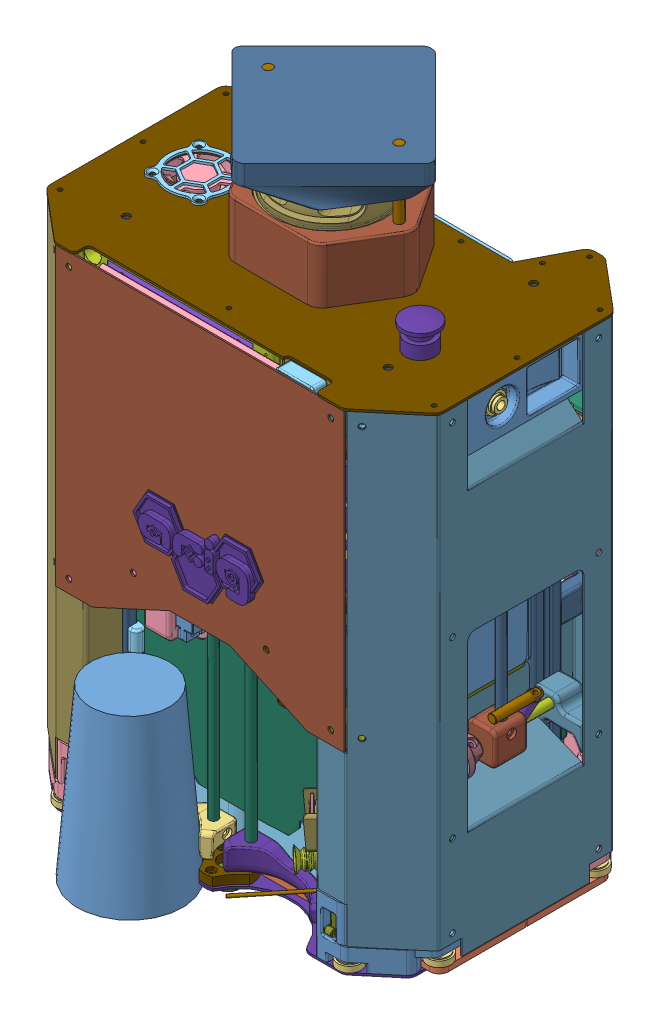
SolidWorks assembly _2021_RobotSecondaire_V1, configuration Default. Lengths in mm.
Overall size (279.45 476 252.7).
311 component instances, 136 part files, 133 mates.
Components (placement in the parent):
- 2020_ADJ_Bouee-1: 2020_ADJ_Bouee [Rouge] at (37.5 0 100) size (72 115 72) (hidden)
- 2020_ADJ_Bouee-2: 2020_ADJ_Bouee [Vert] at (-37.5 0 100) size (72 115 72)
- 2020_ADJ_Bouee-3: 2020_ADJ_Bouee [Rouge] at (37.5 0 -100) size (72 115 72) (hidden)
- 2020_ADJ_Bouee-4: 2020_ADJ_Bouee [Vert] at (-37.5 0 -100) size (72 115 72) (hidden)
- VolumeRobot-1: VolumeRobot [Default] at origin size (270 345 180) (hidden)
- BaseRoulante-1: BaseRoulante [Défaut] at origin size (279.45 126.82 126.23)
  - BaseRoulante_Plaque-1: BaseRoulante_Plaque [Défaut] at (0 7 0) x (1 0 0) z (0 1 0) size (270 120 4)
  - RoulementAngle-3: RoulementAngle [Défaut] at (-128.5 13.75 -53.5) size (16 9.5 16)
  - RoulementAngle-4: RoulementAngle [Défaut] at (-128.5 13.75 53.5) x (-0.613388 0 -0.789782) z (0.789782 0 -0.613388) size (16 9.5 16)
  - BaseRoulante_Codeur-1: BaseRoulante_Codeur [Défaut] at (-117.5 24 0) size (31.5 112 93)
    - Kubler-05.2400.1212.1024-1: Kubler-05.2400.1212.1024 [fil a Drt] at (-9.5 0 0) x (1 0 0) z (0 -0.399238 -0.916848) size (31 88.25 62)
      - Kubler-05.2400.1212.1024-1: Kubler-05.2400.1212.1024 [Défaut] at origin size (31 36 24)
      - Kubler-rayon mini cable-1: Kubler-rayon mini cable [Défaut] at (25 -24 0) x (0 0 -1) z (1 0 0) size (52.25 52.25 4.5) (hidden)
    - Igus_TK_04_09_coulisseau-1: Igus_TK_04_09_coulisseau [Défaut] at (11.5 77 35) x (0 0 1) z (-1 0 0) size (20 29 8.3)
    - Igus_TK_04_09_Rail_L50-1: Igus_TK_04_09_Rail_L50 [Défaut] at (11.5 14.5 -35) x (0 0 1) z (-1 0 0) size (9.6 50 6.3)
    - BaseRoulante_SupportCodeur-1: BaseRoulante_SupportCodeur [Défaut] at (1.5 32.5 0) x (0 0 1) z (-1 0 0) size (93 50 1.5)
    - Igus_TK_04_09_coulisseau-2: Igus_TK_04_09_coulisseau [Défaut] at (11.5 77 -35) x (0 0 1) z (-1 0 0) size (20 29 8.3)
    - Igus_TK_04_09_Rail_L50-2: Igus_TK_04_09_Rail_L50 [Défaut] at (11.5 14.5 35) x (0 0 1) z (-1 0 0) size (9.6 50 6.3)
    - BaseRoulante_RoueCodeuse-1: BaseRoulante_RoueCodeuse [Défaut] at (-7.5 0 0) size (9 48 48)
  - BaseRoulante_Codeur-9: BaseRoulante_Codeur [Défaut] at (117.5 24 0) x (-1 0 0) z (0 0 -1) size (31.5 112 93)
    - Kubler-05.2400.1212.1024-1: Kubler-05.2400.1212.1024 [fil a Drt] at (-9.5 0 0) x (1 0 0) z (0 -0.399238 -0.916848) size (31 88.25 62)
      - Kubler-05.2400.1212.1024-1: Kubler-05.2400.1212.1024 [Défaut] at origin size (31 36 24)
      - Kubler-rayon mini cable-1: Kubler-rayon mini cable [Défaut] at (25 -24 0) x (0 0 -1) z (1 0 0) size (52.25 52.25 4.5) (hidden)
    - Igus_TK_04_09_coulisseau-1: Igus_TK_04_09_coulisseau [Défaut] at (11.5 77 35) x (0 0 1) z (-1 0 0) size (20 29 8.3)
    - Igus_TK_04_09_Rail_L50-1: Igus_TK_04_09_Rail_L50 [Défaut] at (11.5 14.5 -35) x (0 0 1) z (-1 0 0) size (9.6 50 6.3)
    - BaseRoulante_SupportCodeur-1: BaseRoulante_SupportCodeur [Défaut] at (1.5 32.5 0) x (0 0 1) z (-1 0 0) size (93 50 1.5)
    - Igus_TK_04_09_coulisseau-2: Igus_TK_04_09_coulisseau [Défaut] at (11.5 77 -35) x (0 0 1) z (-1 0 0) size (20 29 8.3)
    - Igus_TK_04_09_Rail_L50-2: Igus_TK_04_09_Rail_L50 [Défaut] at (11.5 14.5 35) x (0 0 1) z (-1 0 0) size (9.6 50 6.3)
    - BaseRoulante_RoueCodeuse-1: BaseRoulante_RoueCodeuse [Défaut] at (-7.5 0 0) size (9 48 48)
  - BaseRoulante_BlocMoteur-1: BaseRoulante_BlocMoteur [Défaut] at (-64.5 31 0) x (0 0 1) z (1 0 0) size (94.63 94.63 89.1)
    - 2232U_SR.stp-1: 2232U_SR.stp [Défaut] at (0 0 55.6) x (-0.975053 0.221972 0) z (0 0 -1) size (22 22 44.5)
    - 20-1R_flange_b.stp-1: 20-1R_flange_b.stp [Défaut] at (0 0 23.4) x (-0.97442 0.224736 0) z (0 0 -1) size (20 20 10.5)
    - 20-1R_2stage.stp-1: 20-1R_2stage.stp [Défaut] x (-1 0 0) z (0 0 -1) size (20 20 32.7)
    - RoueMotrice-1: RoueMotrice [Défaut] at (-257.7357 446.4113 -14.3) x (-0.5 0.866025 0) z (0 0 -1) size (69.28 69.28 30)
      - Pneu-1: Pneu [Défaut] at (-515.4714 0 -15) size (64 64 30)
      - Jante-1: Jante [Défaut] at (-515.4714 0 15) x (-0.834512 -0.55099 0) z (0 0 1) size (50 50 30)
    - BaseRoulante_CoupleurMoteur-1: BaseRoulante_CoupleurMoteur [Défaut] at (0 0 -22.3) x (0 -1 0) z (-1 0 0) size (12 18 13.86)
  - BaseRoulante_Carter-1: BaseRoulante_Carter [Défaut] at (-106 38.5 27.5) size (43.05 55 12.4)
  - BaseRoulante_Carter-3: BaseRoulante_Carter [Défaut] at (-106 38.5 -27.5) x (1 0 0) z (0 0 -1) size (43.05 55 12.4)
  - BaseRoulante_ToleCarter-1: BaseRoulante_ToleCarter [Défaut] at (-61 66 0) x (0 0 1) z (-1 0 0) size (80 1.5 51)
  - RoulementAngle-5: RoulementAngle [Défaut] at (128.5 13.75 -53.5) x (-1 0 0) z (0 0 -1) size (16 9.5 16)
  - RoulementAngle-6: RoulementAngle [Défaut] at (128.5 13.75 53.5) x (0.613388 0 -0.789782) z (0.789782 0 0.613388) size (16 9.5 16)
  - BaseRoulante_Carter-4: BaseRoulante_Carter [Défaut] at (106 38.5 27.5) x (-1 0 0) z (0 0 1) size (43.05 55 12.4)
  - BaseRoulante_ToleCarter-2: BaseRoulante_ToleCarter [Défaut] at (61 66 0) x (0 0 -1) z (1 0 0) size (80 1.5 51)
  - BaseRoulante_BlocMoteur-2: BaseRoulante_BlocMoteur [Défaut] at (64.5 31 0) x (0 0 1) z (-1 0 0) size (94.63 94.63 89.1)
    - 2232U_SR.stp-1: 2232U_SR.stp [Défaut] at (0 0 55.6) x (-0.975053 0.221972 0) z (0 0 -1) size (22 22 44.5)
    - 20-1R_flange_b.stp-1: 20-1R_flange_b.stp [Défaut] at (0 0 23.4) x (-0.97442 0.224736 0) z (0 0 -1) size (20 20 10.5)
    - 20-1R_2stage.stp-1: 20-1R_2stage.stp [Défaut] x (-1 0 0) z (0 0 -1) size (20 20 32.7)
    - RoueMotrice-1: RoueMotrice [Défaut] at (-257.7357 446.4113 -14.3) x (-0.5 0.866025 0) z (0 0 -1) size (69.28 69.28 30)
      - Pneu-1: Pneu [Défaut] at (-515.4714 0 -15) size (64 64 30)
      - Jante-1: Jante [Défaut] at (-515.4714 0 15) x (-0.834512 -0.55099 0) z (0 0 1) size (50 50 30)
    - BaseRoulante_CoupleurMoteur-1: BaseRoulante_CoupleurMoteur [Défaut] at (0 0 -22.3) x (0 -1 0) z (-1 0 0) size (12 18 13.86)
  - BaseRoulante_Carter-5: BaseRoulante_Carter [Défaut] at (106 38.5 -27.5) x (-1 0 0) z (0 0 -1) size (43.05 55 12.4)
  - BlocSuppMoteur2021-1: BlocSuppMoteur2021 [Default] at (-52 31 0) x (-1 0 0) z (0 0 -1) size (52.39 39.47 48.92)
  - BlocSuppMoteur2021-2: BlocSuppMoteur2021 [Default] at (52 31 0) size (52.39 39.47 48.92)
- BlocSup-1: BlocSup [Défaut] at (0 -2.5 0) size (270 207.07 197.32)
  - BlocSup_Plaque-1: BlocSup_Plaque [Défaut] at (0 343.5 0) x (0 0 -1) z (1 0 0) size (180 1.5 270)
  - BlocSup_CarterGauche-1: BlocSup_CarterGauche [Défaut] at (135 295.5187 -42.1103) x (0 0 -1) z (1 0 0) size (173.26 35 33.94)
  - BlocSup_CarterDroite-1: BlocSup_CarterDroite [Défaut] at (-135 308.5 0) x (0 0 1) z (-1 0 0) size (173.26 35 33.94)
  - BlocSup_Charniere-1: BlocSup_Charniere [Défaut] at (0 238 -83.5) x (0 0 -1) z (1 0 0) size (10 17.5 158)
  - BlocSup_SupportCharniere-1: BlocSup_SupportCharniere [Défaut] at (-90 227.5 -50) x (-1 0 0) z (0 0 -1) size (29 18 30)
  - BlocSup_SupportEcran-1: BlocSup_SupportEcran [Défaut] at (0 292.3655 -56.8959) x (-1 0 0) z (0 0.32983 -0.94404) size (138 106.19 17.63)
  - BlocSup_CarterEcran-1: BlocSup_CarterEcran [Défaut] at (70.0918 245.5 -90) x (-1 0 0) z (0 0 -1) size (29.48 98 45)
  - _Symétrie_BlocSup_CarterEcran-1: _Symétrie_BlocSup_CarterEcran [Défaut] at (-70.0918 245.5 -90) size (29.48 98 45.96)
  - Lidar-1: Lidar [Default] at (0 345 0) size (135.87 85 134.45)
    - Lidar_Base-1: Lidar_Base [Défaut] at origin size (105 35.5 75)
    - Lidar_Tige-1: Lidar_Tige [Défaut] at (-45 5 -2.5) size (6 80 6)
    - Lidar_Tige-2: Lidar_Tige [Défaut] at (45 5 -2.5) size (6 80 6)
    - Lidar_Top-1: Lidar_Top [Défaut] at (0 85 -2.5) x (-1 0 0) z (0 0 1) size (135.87 27.01 134.45)
    - Lidar_Cache-1: Lidar_Cache [Défaut] at (0 38.3 -2.5) x (-1 0 0) z (0 0 1) size (110 38.3 83)
    - rplidar-a2-1: rplidar-a2 [Défaut] at (-75 9.2861 -6.0269) x (0 0 -1) z (1 0 0) size (80.61 40.81 84.84)
  - Tirette-1: Tirette [Défaut] at (15.8155 -23.9188 -0.5) size (18.01 65.48 50.46)
    - TiretteDiam6-1: TiretteDiam6 [Default] at (-106.1573 340.7878 -102.5731) x (-0.007647 0.642769 0.766022) z (0 -0.766044 0.642788) size (6 6 61)
    - Tirette_Support-1: Tirette_Support [Défaut] at (-106.1573 276.0497 -60) x (0 0 1) z (-1 0 0) size (28.63 58.34 18.1)
    - microswitchGaletAss-1: microswitchGaletAss [Défaut] at (-106.1573 330.3845 -72.9571) x (0 -0.766044 0.642788) z (1 0 0) size (21.06 21.1 7)
      - microswitchGalet02-1: microswitchGalet02 [Défaut] at origin size (20 15 7)
      - microswitchGalet01-1: microswitchGalet01 [Défaut] at (1.7099 12.1145 0) x (0.996636 -0.081957 0) z (0 0 1) size (19 9 6)
  - APEM_A01ES_A0154B-1: APEM_A01ES_A0154B [Défaut] at (90 345 28) size (24 61 24)
  - Ecran_5po_DFR0550-1: Ecran_5po_DFR0550 [Default] at (0 297.1481 -70.5845) x (1 0 0) z (0 0.32983 -0.94404) size (121 76 27.3)
  - interrupteur principal-1: interrupteur principal [Défaut] at (121.5 326 -20) x (0 0 1) z (0 1 0) size (32 33.35 25)
  - _Symétrie_BlocSup_SupportCharniere-3: _Symétrie_BlocSup_SupportCharniere [Défaut] at (90 227.5 -50) size (29 18 30)
  - PriseJackAlim-1: PriseJackAlim [Default] at (123.5 326 15) x (0 -1 0) z (0 0 1) size (16.17 25.3 16)
  - Ventilo_AAB_Diam40-1: Ventilo_AAB_Diam40 [Défaut] at (-90 333.5 0) x (1 0 0) z (0 1 0) size (45 40 10)
  - Ventilo_Cache-1: Ventilo_Cache [Défaut] at (-90 345 0) x (0 0 -1) z (1 0 0) size (42.6 1.5 42.6)
  - Raspberry-Pi-4-Model-B-03-1: Raspberry-Pi-4-Model-B-03 [Défaut] at (-32.5 266.2952 -67.1696) x (1 0 0) z (0 -0.32983 0.94404) size (87.94 57.9 19.63)
  - InterfaceRaspi-1: InterfaceRaspi [Défaut] at (-107.5 400.9752 -9.9988) x (1 0 0) z (0 -0.32983 0.94404) size (65 56 17.8)
  - 4010 - Blower Assembly-1: 4010 - Blower Assembly [Défaut] at (19.1478 275.9461 -78.4041) x (-1 0 0) z (0 -0.32983 0.94404) size (40 40 9.75)
  - Ventilo_Raspi_Support-1: Ventilo_Raspi_Support [Défaut] at (0 270.259 -67.9033) x (-1 0 0) z (0 0.94404 0.32983) size (64 15.5 14.5)
- ProfiléX20_330-1: ProfiléX20_330 [Défaut] at (80 11 -40) x (1 0 0) z (0 1 0) size (20 20 330)
- ProfiléX20_330-2: ProfiléX20_330 [Défaut] at (-100 11 -40) x (1 0 0) z (0 1 0) size (20 20 330)
- ProfiléX20_330-3: ProfiléX20_330 [Défaut] at (-100 11 60) x (1 0 0) z (0 1 0) size (20 20 330)
- ProfiléX20_330-4: ProfiléX20_330 [Défaut] at (100 11 60) x (0 0 -1) z (0 1 0) size (20 20 330)
- BrasLateral-1: BrasLateral [Default] at (-82 117.5 38.35) x (-1 0 0) z (0 0 -1) size (52.5 125.87 147.5)
  - Access_HS-645_Rond-1: Access_HS-645_Rond [Défaut] at (28 -10.2 7.8) x (-0.986286 0.165048 0) z (0.165048 0.986286 0) size (24 5 24)
  - Servo_HS-485-HB-1: Servo_HS-485-HB [Default] at (28 -10.2 -31.94) x (-1 0 0) z (0 0 1) size (19.81 54.15 42.74)
  - Bras_AxePivot-1: Bras_AxePivot [Default] at (28 -10.2 16.3) x (0.492424 0.870356 0) z (0 0 1) size (6 6 80)
  - Bras_Alu_TubeCarre_07.5-1: Bras_Alu_TubeCarre_07.5 [Default] at (34.6477 1.5498 55.3) x (-0.870356 0.492424 0) z (-0.492424 -0.870356 0) size (8 8 26)
  - Bras_AxeButee-1: Bras_AxeButee [Default] at (41.2954 13.2996 59.3) x (0.492424 0.870356 0) z (0 0 -1) size (6 6 33)
  - Bras_Rouleau-1: Bras_Rouleau [Default] at (35.2953 -10.2 38.75) x (0 0 1) z (0 1 0) size (24.5 22.96 102.46)
    - Bras_Axe-1: Bras_Axe [Default] at origin size (6 6 94)
    - Bras_Pivot-1: Bras_Pivot [Default] at (0 0 -8) x (0 1 0) z (1 0 0) size (22.5 23 22.5)
    - Igus_Bague_d06-1: Igus_Bague_d06 [Défaut] at (-12.25 -7.2953 0) size (10 12 12)
    - Igus_Bague_d06-2: Igus_Bague_d06 [Défaut] at (12.25 -7.2953 0) x (-1 0 0) z (0 -0.759835 -0.650115) size (10 12 12)
  - Bras_FixAxePivot-1: Bras_FixAxePivot [Défaut] at (28 -10.2 12.3) x (-0.870356 0.492424 0) z (0.492424 0.870356 0) size (24 14 24)
  - Bras_SupportAxe-1: Bras_SupportAxe [Défaut] at (18 -21.2 88.35) x (0 0 1) z (1 0 0) size (18 26 35)
  - Bras_SupportServo_Bottom-1: Bras_SupportServo_Bottom [Défaut] at (8 -42.065 -11.65) x (0 0 -1) z (1 0 0) size (18 22 35)
  - Bras_SupportServo_Top-1: Bras_SupportServo_Top [Défaut] at (8 19.815 -11.65) x (-1 0 0) z (0 0 -1) size (39 18 44.5)
- Pneumatique-6: Pneumatique [Défaut] at (-90 67.5 0) size (98.5 73.06 104.94) (hidden)
  - CroixPiquageRapideD06-1: CroixPiquageRapideD06 [Default] at (39.5 20.5 0) x (0 0 1) z (0 -1 0) size (38 38 13)
  - CapteurVide_CKD_PPE-V01A-H6-B-1: CapteurVide_CKD_PPE-V01A-H6-B [Défaut] at (63 20.5 0) x (0 -0.999843 0.017733) z (0 0.017733 0.999843) size (37 43 15)
  - Electrovanne_CylindriqueD24_NC_12V-1: Electrovanne_CylindriqueD24_NC_12V [Default] at (-8.5 14 26) x (0 0.999367 0.035582) z (0 0.035582 -0.999367) size (38.24 53 24.48)
  - Electrovanne_CylindriqueD24_NC_12V-2: Electrovanne_CylindriqueD24_NC_12V [Default] at (-8.5 14 -26) x (0 0.999176 0.040592) z (0 0.040592 -0.999176) size (38.24 53 24.48)
  - CroixPiquageRapideD06-2: CroixPiquageRapideD06 [Default] at (39.5 37.5 0) x (0 0 1) z (0 -1 0) size (38 38 13)
  - CapteurVide_CKD_PPE-V01A-H6-B-2: CapteurVide_CKD_PPE-V01A-H6-B [Défaut] at (63 37.5 0) x (0 0.007638 -0.999971) z (0 -0.999971 -0.007638) size (37 43 15)
  - Pneumatique_Support-1: Pneumatique_Support [Défaut] at origin size (64.23 14 83)
  - Pneumatique_Top-1: Pneumatique_Top [Défaut] at (0 15 0) size (19.23 27.5 83)
  - Pneumatique_Entretoise-1: Pneumatique_Entretoise [Défaut] at (39.5 27 0) size (24 4 24)
  - tuyau1^Pneumatique-1: tuyau1^Pneumatique [Défaut] at (20.5 37.5 0) x (0 0 1) z (-1 0 0) size (31.4 24.42 35.33) (virtual)
  - tuyau2^Pneumatique-1: tuyau2^Pneumatique [Défaut] at (20.5 20.5 0) x (0 0 1) z (-1 0 0) size (33.54 37.08 42) (virtual)
  - tuyau3^Pneumatique-1: tuyau3^Pneumatique [Défaut] at (39.5 20.5 -19) x (0 -1 0) z (0 0 -1) size (42.15 12.06 47.59) (virtual)
  - tuyau4^Pneumatique-1: tuyau4^Pneumatique [Défaut] at (39.5 37.5 -19) x (0 -1 0) z (0 0 -1) size (49.1 26.51 49.11) (virtual)
  - tuyau5^Pneumatique-1: tuyau5^Pneumatique [Défaut] at (39.5 20.5 19) x (0 1 0) z (0 0 1) size (32.28 26.54 48.84) (virtual)
  - tuyau6^Pneumatique-1: tuyau6^Pneumatique [Défaut] at (39.5 37.5 19) x (0 1 0) z (0 0 1) size (59 12.1 47.35) (virtual)
- Pneumatique-7: Pneumatique [Défaut] at (90 67.5 0) x (-1 0 0) z (0 0 -1) size (98.5 73.06 104.94) (hidden)
  - CroixPiquageRapideD06-1: CroixPiquageRapideD06 [Default] at (39.5 20.5 0) x (0 0 1) z (0 -1 0) size (38 38 13)
  - CapteurVide_CKD_PPE-V01A-H6-B-1: CapteurVide_CKD_PPE-V01A-H6-B [Défaut] at (63 20.5 0) x (0 -0.999843 0.017733) z (0 0.017733 0.999843) size (37 43 15)
  - Electrovanne_CylindriqueD24_NC_12V-1: Electrovanne_CylindriqueD24_NC_12V [Default] at (-8.5 14 26) x (0 0.999367 0.035582) z (0 0.035582 -0.999367) size (38.24 53 24.48)
  - Electrovanne_CylindriqueD24_NC_12V-2: Electrovanne_CylindriqueD24_NC_12V [Default] at (-8.5 14 -26) x (0 0.999176 0.040592) z (0 0.040592 -0.999176) size (38.24 53 24.48)
  - CroixPiquageRapideD06-2: CroixPiquageRapideD06 [Default] at (39.5 37.5 0) x (0 0 1) z (0 -1 0) size (38 38 13)
  - CapteurVide_CKD_PPE-V01A-H6-B-2: CapteurVide_CKD_PPE-V01A-H6-B [Défaut] at (63 37.5 0) x (0 0.007638 -0.999971) z (0 -0.999971 -0.007638) size (37 43 15)
  - Pneumatique_Support-1: Pneumatique_Support [Défaut] at origin size (64.23 14 83)
  - Pneumatique_Top-1: Pneumatique_Top [Défaut] at (0 15 0) size (19.23 27.5 83)
  - Pneumatique_Entretoise-1: Pneumatique_Entretoise [Défaut] at (39.5 27 0) size (24 4 24)
  - tuyau1^Pneumatique-1: tuyau1^Pneumatique [Défaut] at (20.5 37.5 0) x (0 0 1) z (-1 0 0) size (31.4 24.42 35.33) (virtual)
  - tuyau2^Pneumatique-1: tuyau2^Pneumatique [Défaut] at (20.5 20.5 0) x (0 0 1) z (-1 0 0) size (33.54 37.08 42) (virtual)
  - tuyau3^Pneumatique-1: tuyau3^Pneumatique [Défaut] at (39.5 20.5 -19) x (0 -1 0) z (0 0 -1) size (42.15 12.06 47.59) (virtual)
  - tuyau4^Pneumatique-1: tuyau4^Pneumatique [Défaut] at (39.5 37.5 -19) x (0 -1 0) z (0 0 -1) size (49.1 26.51 49.11) (virtual)
  - tuyau5^Pneumatique-1: tuyau5^Pneumatique [Défaut] at (39.5 20.5 19) x (0 1 0) z (0 0 1) size (32.28 26.54 48.84) (virtual)
  - tuyau6^Pneumatique-1: tuyau6^Pneumatique [Défaut] at (39.5 37.5 19) x (0 1 0) z (0 0 1) size (59 12.1 47.35) (virtual)
- Pneumatique2-1: Pneumatique2 [Défaut] at (80 92 0) x (0 0 1) z (-1 0 0) size (118 63.5 92.8)
  - Pneumatique_Support2-1: Pneumatique_Support2 [Défaut] at (0 0 -10) size (118 15 27.1)
  - CroixPiquageRapideD06-1: CroixPiquageRapideD06 [Default] at (12.5 14.5 29.25) x (-1 0 0) z (0 -1 0) size (38 38 13)
  - CroixPiquageRapideD06-2: CroixPiquageRapideD06 [Default] at (-12.5 -6.5 29.25) x (1 0 0) z (0 1 0) size (38 38 13)
  - CapteurVide_CKD_PPE-V01A-H6-B-1: CapteurVide_CKD_PPE-V01A-H6-B [Défaut] at (12.5 14.5 52.75) x (0 -1 0) z (-1 0 0) size (37 43 15)
  - CapteurVide_CKD_PPE-V01A-H6-B-2: CapteurVide_CKD_PPE-V01A-H6-B [Défaut] at (-12.5 -6.5 52.75) x (0 1 0) z (1 0 0) size (37 43 15)
  - Electrovanne_CylindriqueD24_NC_12V-1: Electrovanne_CylindriqueD24_NC_12V [Default] at (12.5 -18.5 -2) x (0 0 1) z (-1 0 0) size (38.24 53 24.48)
  - Electrovanne_CylindriqueD24_NC_12V-2: Electrovanne_CylindriqueD24_NC_12V [Default] at (-12.5 26.5 -2) x (0 0 1) z (1 0 0) size (38.24 53 24.48)
  - Pneumatique_Fix-1: Pneumatique_Fix [Défaut] at (0 0 -2) x (-1 0 0) z (0 0 -1) size (75 8 14.55)
  - Pièce4^Pneumatique2-1: Pièce4^Pneumatique2 [Défaut] at (-9 -6.5 29.25) x (0 -1 0) z (1 0 0) size (24.78 14.3 44.64) (virtual)
  - Pièce5^Pneumatique2-1: Pièce5^Pneumatique2 [Défaut] at (16 14.5 29.25) x (0 -1 0) z (1 0 0) size (50.6 27.61 36.51) (virtual)
  - Pièce6^Pneumatique2-1: Pièce6^Pneumatique2 [Défaut] at (-16 -6.5 29.25) x (0 1 0) z (-1 0 0) size (29.52 27.83 36.35) (virtual)
  - Pièce7^Pneumatique2-1: Pièce7^Pneumatique2 [Défaut] at (9 14.5 29.25) x (0 1 0) z (-1 0 0) size (45.5 14.26 63.44) (virtual)
- Tole_Centre-5: Tole_Centre [Défaut] at (0 153.5 -38.5) x (1 0 0) z (0 0 -1) size (196 55 1.5)
- Tole_Centre-6: Tole_Centre [Défaut] at (0 153.5 40) x (1 0 0) z (0 0 -1) size (196 55 1.5)
- PouseGobelet-3: PouseGobelet [Défaut] at (1 9.5363 0) x (-1 0 0) z (0 0 -1) size (70.57 166.01 48.5)
  - PouseGobelet_Tige-1: PouseGobelet_Tige [Default] at (13.938 11.9952 67.12) x (-1 0 0) z (0 1 0) size (6 6 154)
  - PouseGobelet_CoupleurServo-1: PouseGobelet_CoupleurServo [Défaut] at (18.938 153.9952 58.12) x (0 -1 0) z (0 0 -1) size (24 16.5 26)
  - PouseGobelet_Fourche-1: PouseGobelet_Fourche [Défaut] at (38.938 5.9952 101.12) size (68.64 17.55 22.57)
  - PouseGobelet_SupportServo-1: PouseGobelet_SupportServo [Défaut] at (37.7 143.9637 68) x (0 0 -1) z (1 0 0) size (48.5 55 18)
  - Access_HS-645_Rond-1: Access_HS-645_Rond [Défaut] at (23.438 153.9952 58.12) x (0 0.939693 -0.34202) z (0 0.34202 0.939693) size (24 5 24)
  - Servo_HS-645-MG_2-1: Servo_HS-645-MG_2 [Défaut] at (62.936 123.7692 48.341) x (0 0 1) z (0 -1 0) size (19.56 43.24 53.34)
- _Symétrie_PouseGobelet-3: _Symétrie_PouseGobelet [Défaut] at (-1 9.5363 0) size (70.57 166.01 48.5)
  - PouseGobelet_Tige-1: PouseGobelet_Tige [Default] at (13.938 11.9952 -67.12) x (1 0 0) z (0 1 0) size (6 6 154)
  - _Symétrie_PouseGobelet_CoupleurServo-1: _Symétrie_PouseGobelet_CoupleurServo [Défaut] at (18.938 153.9952 -58.12) x (0 -1 0) z (0 0 -1) size (24 16.5 26)
  - _Symétrie_PouseGobelet_Fourche-1: _Symétrie_PouseGobelet_Fourche [Défaut] at (38.938 5.9952 -101.12) size (68.64 17.55 22.57)
  - _Symétrie_PouseGobelet_SupportServo-1: _Symétrie_PouseGobelet_SupportServo [Défaut] at (37.7 143.9637 -68) x (0 0 1) z (-1 0 0) size (48.5 55 18)
  - Access_HS-645_Rond-1: Access_HS-645_Rond [Défaut] at (23.438 153.9952 -58.12) x (0 0.939693 -0.34202) z (0 0.34202 0.939693) size (24 5 24)
  - Servo_HS-645-MG_2-2: Servo_HS-645-MG_2 [Défaut] at (62.936 123.7692 -67.899) x (0 0 1) z (0 -1 0) size (19.56 43.24 53.34)
- PouseGobelet-1: PouseGobelet [Défaut] at (-1 9.5363 0) size (70.57 166.01 48.5)
  - PouseGobelet_Tige-1: PouseGobelet_Tige [Default] at (13.938 11.9952 67.12) x (-1 0 0) z (0 1 0) size (6 6 154)
  - PouseGobelet_CoupleurServo-1: PouseGobelet_CoupleurServo [Défaut] at (18.938 153.9952 58.12) x (0 -1 0) z (0 0 -1) size (24 16.5 26)
  - PouseGobelet_Fourche-1: PouseGobelet_Fourche [Défaut] at (38.938 5.9952 101.12) size (68.64 17.55 22.57)
  - PouseGobelet_SupportServo-1: PouseGobelet_SupportServo [Défaut] at (37.7 143.9637 68) x (0 0 -1) z (1 0 0) size (48.5 55 18)
  - Access_HS-645_Rond-1: Access_HS-645_Rond [Défaut] at (23.438 153.9952 58.12) x (0 0.939693 -0.34202) z (0 0.34202 0.939693) size (24 5 24)
  - Servo_HS-645-MG_2-1: Servo_HS-645-MG_2 [Défaut] at (62.936 123.7692 48.341) x (0 0 1) z (0 -1 0) size (19.56 43.24 53.34)
- _Symétrie_PouseGobelet-4: _Symétrie_PouseGobelet [Défaut] at (1 9.5363 0) x (-1 0 0) z (0 0 -1) size (70.57 166.01 48.5)
  - PouseGobelet_Tige-1: PouseGobelet_Tige [Default] at (13.938 11.9952 -67.12) x (1 0 0) z (0 1 0) size (6 6 154)
  - _Symétrie_PouseGobelet_CoupleurServo-1: _Symétrie_PouseGobelet_CoupleurServo [Défaut] at (18.938 153.9952 -58.12) x (0 -1 0) z (0 0 -1) size (24 16.5 26)
  - _Symétrie_PouseGobelet_Fourche-1: _Symétrie_PouseGobelet_Fourche [Défaut] at (38.938 5.9952 -101.12) size (68.64 17.55 22.57)
  - _Symétrie_PouseGobelet_SupportServo-1: _Symétrie_PouseGobelet_SupportServo [Défaut] at (37.7 143.9637 -68) x (0 0 1) z (-1 0 0) size (48.5 55 18)
  - Access_HS-645_Rond-1: Access_HS-645_Rond [Défaut] at (23.438 153.9952 -58.12) x (0 0.939693 -0.34202) z (0 0.34202 0.939693) size (24 5 24)
  - Servo_HS-645-MG_2-2: Servo_HS-645-MG_2 [Défaut] at (62.936 123.7692 -67.899) x (0 0 1) z (0 -1 0) size (19.56 43.24 53.34)
- PompeVide-AirpoD2028B-12vdc-1: PompeVide-AirpoD2028B-12vdc [Défaut] at (-19.3 12 40.3) x (0 0 -1) z (0 1 0) size (38.6 62.4 92)
- PompeVide-AirpoD2028B-12vdc-2: PompeVide-AirpoD2028B-12vdc [Défaut] at (19.3 12 40.3) x (0 0 1) z (0 1 0) size (38.6 62.4 92)
- BlocVentouse-1: BlocVentouse [Défaut] at (90 24 50) size (59.95 59 74.7)
  - BlocVentouse_SupportVentouse-1: BlocVentouse_SupportVentouse [Défaut] at (-52.5 0 50) size (36.21 32 31.1)
  - Ventouse_MP-S15_L16-1: Ventouse_MP-S15_L16 [Default] at (-25.3134 22 16.4273) x (0 -1 0) z (-0.777146 0 -0.62932) size (15 16 15)
  - Pololu capteur-1: Pololu capteur [Default] at (-6.4473 0 20.3813) x (0 1 0) z (-0.62932 0 0.777146) size (30.1 9 61.8)
    - pololu gp2y0d805-1: pololu gp2y0d805 [Défaut] at origin size (30.1 9 11.8)
    - faisceau pololu gp2y0d-1: faisceau pololu gp2y0d [5cm] at (12 4.5 9.6) size (2 2 50)
  - EmboutVentouse_Droit_D7D5-1: EmboutVentouse_Droit_D7D5 [Default] at (-24.8099 22 15.8056) x (0.777146 0 0.62932) z (0 -1 0) size (8 12 9.24)
  - EmboutVentouse_Droit_D7D5_2-1: EmboutVentouse_Droit_D7D5_2 [Default] at (-18 32 -1) x (0 1 0) z (0 0 -1) size (15.2 8.1 8.1)
  - BlocVentouse_SupportCapteurCouleur-1: BlocVentouse_SupportCapteurCouleur [Défaut] at (-52.5 37 50) size (48.3 22.13 28.3)
  - ADAFRUIT_tcs34725_rgb_sensor-1: ADAFRUIT_tcs34725_rgb_sensor [Default] at (-26.4624 47.3219 23.8132) x (0.061386 -0.996919 -0.04883) z (-0.70659 -0.008851 -0.707568) size (20.51 3 20.51)
- _Symétrie_BlocVentouse-3: _Symétrie_BlocVentouse [Défaut] at (-90 24 50) x (-1 0 0) z (0 0 -1) size (59.95 59 74.7)
  - _Symétrie_BlocVentouse_SupportVentouse-1: _Symétrie_BlocVentouse_SupportVentouse [Défaut] at (-52.5 0 -50) size (36.21 32 31.1)
  - Ventouse_MP-S15_L16-1: Ventouse_MP-S15_L16 [Default] at (-25.3134 22 -16.4273) x (0 -1 0) z (0.777146 0 -0.62932) size (15 16 15)
  - Pololu capteur-1: Pololu capteur [Default] at (-13.4416 0 -14.7174) x (0 1 0) z (-0.62932 0 -0.777146) size (30.1 9 61.8)
    - pololu gp2y0d805-1: pololu gp2y0d805 [Défaut] at origin size (30.1 9 11.8)
    - faisceau pololu gp2y0d-1: faisceau pololu gp2y0d [5cm] at (12 4.5 9.6) size (2 2 50)
  - EmboutVentouse_Droit_D7D5-1: EmboutVentouse_Droit_D7D5 [Default] at (-24.8099 22 -15.8056) x (0.388573 0.866025 -0.31466) z (-0.673028 0.5 0.545007) size (8 12 9.24)
  - EmboutVentouse_Droit_D7D5_2-1: EmboutVentouse_Droit_D7D5_2 [Default] at (-18 32 1) x (0 1 0) z (-0.777146 0 0.62932) size (15.2 8.1 8.1)
  - _Symétrie_BlocVentouse_SupportCapteurCouleur-1: _Symétrie_BlocVentouse_SupportCapteurCouleur [Défaut] at (-52.5 37 -50) size (48.3 22.13 28.3)
  - ADAFRUIT_tcs34725_rgb_sensor-1: ADAFRUIT_tcs34725_rgb_sensor [Default] at (-26.3889 47.6196 -23.9197) x (0.049876 -0.996931 0.060341) z (0.707495 -0.007378 -0.70668) size (20.51 3 20.51)
- BlocVentouse-2: BlocVentouse [Défaut] at (-90 24 -50) x (-1 0 0) z (0 0 -1) size (59.95 59 74.7)
  - BlocVentouse_SupportVentouse-1: BlocVentouse_SupportVentouse [Défaut] at (-52.5 0 50) size (36.21 32 31.1)
  - Ventouse_MP-S15_L16-1: Ventouse_MP-S15_L16 [Default] at (-25.3134 22 16.4273) x (0 -1 0) z (-0.777146 0 -0.62932) size (15 16 15)
  - Pololu capteur-1: Pololu capteur [Default] at (-6.4473 0 20.3813) x (0 1 0) z (-0.62932 0 0.777146) size (30.1 9 61.8)
    - pololu gp2y0d805-1: pololu gp2y0d805 [Défaut] at origin size (30.1 9 11.8)
    - faisceau pololu gp2y0d-1: faisceau pololu gp2y0d [5cm] at (12 4.5 9.6) size (2 2 50)
  - EmboutVentouse_Droit_D7D5-1: EmboutVentouse_Droit_D7D5 [Default] at (-24.8099 22 15.8056) x (0.777146 0 0.62932) z (0 -1 0) size (8 12 9.24)
  - EmboutVentouse_Droit_D7D5_2-1: EmboutVentouse_Droit_D7D5_2 [Default] at (-18 32 -1) x (0 1 0) z (0 0 -1) size (15.2 8.1 8.1)
  - BlocVentouse_SupportCapteurCouleur-1: BlocVentouse_SupportCapteurCouleur [Défaut] at (-52.5 37 50) size (48.3 22.13 28.3)
  - ADAFRUIT_tcs34725_rgb_sensor-1: ADAFRUIT_tcs34725_rgb_sensor [Default] at (-26.4624 47.3219 23.8132) x (0.061386 -0.996919 -0.04883) z (-0.70659 -0.008851 -0.707568) size (20.51 3 20.51)
- _Symétrie_BlocVentouse-4: _Symétrie_BlocVentouse [Défaut] at (90 24 -50) size (59.95 59 74.7)
  - _Symétrie_BlocVentouse_SupportVentouse-1: _Symétrie_BlocVentouse_SupportVentouse [Défaut] at (-52.5 0 -50) size (36.21 32 31.1)
  - Ventouse_MP-S15_L16-1: Ventouse_MP-S15_L16 [Default] at (-25.3134 22 -16.4273) x (0 -1 0) z (0.777146 0 -0.62932) size (15 16 15)
  - Pololu capteur-1: Pololu capteur [Default] at (-13.4416 0 -14.7174) x (0 1 0) z (-0.62932 0 -0.777146) size (30.1 9 61.8)
    - pololu gp2y0d805-1: pololu gp2y0d805 [Défaut] at origin size (30.1 9 11.8)
    - faisceau pololu gp2y0d-1: faisceau pololu gp2y0d [5cm] at (12 4.5 9.6) size (2 2 50)
  - EmboutVentouse_Droit_D7D5-1: EmboutVentouse_Droit_D7D5 [Default] at (-24.8099 22 -15.8056) x (0.388573 0.866025 -0.31466) z (-0.673028 0.5 0.545007) size (8 12 9.24)
  - EmboutVentouse_Droit_D7D5_2-1: EmboutVentouse_Droit_D7D5_2 [Default] at (-18 32 1) x (0 1 0) z (-0.777146 0 0.62932) size (15.2 8.1 8.1)
  - _Symétrie_BlocVentouse_SupportCapteurCouleur-1: _Symétrie_BlocVentouse_SupportCapteurCouleur [Défaut] at (-52.5 37 -50) size (48.3 22.13 28.3)
  - ADAFRUIT_tcs34725_rgb_sensor-1: ADAFRUIT_tcs34725_rgb_sensor [Default] at (-26.3889 47.6196 -23.9197) x (0.049876 -0.996931 0.060341) z (0.707495 -0.007378 -0.70668) size (20.51 3 20.51)
- PompeVide-AirpoD2028B-12vdc-3: PompeVide-AirpoD2028B-12vdc [Défaut] at (-19.3 12 -40.3) x (0 0 -1) z (0 1 0) size (38.6 62.4 92)
- PompeVide-AirpoD2028B-12vdc-4: PompeVide-AirpoD2028B-12vdc [Défaut] at (19.3 12 -40.3) x (0 0 1) z (0 1 0) size (38.6 62.4 92)
- Batterie-2: Batterie [Défaut] at (-98 126 38.25) size (210.28 68.5 76.97)
  - Batterie_Logement_Bottom-1: Batterie_Logement_Bottom [Défaut] at origin size (196 7 76.97)
  - Batterie_Logement_Top-2: Batterie_Logement_Top [Défaut] at (0 55 -76.5) x (1 0 0) z (0 0 -1) size (196 20 76.97)
  - Batterie_Logement_Side-1: Batterie_Logement_Side [Défaut] at (2 27.5 -38.25) x (0 0 -1) z (1 0 0) size (76.5 55.5 2)
  - batterie_logement_porte-1: batterie_logement_porte [Défaut] at (194.1093 27.2584 -38.25) x (0 0 -1) z (0.999991 -0.004328 0) size (69 68 4)
  - Batterie_Logement_VisAMain-1: Batterie_Logement_VisAMain [Défaut] at (196.251 59.9995 -54.25) x (0.001572 0.363339 -0.931656) z (-0.004032 -0.931647 -0.363342) size (11.89 14 11.89)
  - batterieLIPO-1: batterieLIPO [Défaut] at (19.922 9.881 -66.3581) x (0.999954 0 0.009631) z (0 -1 0) size (160 49 34)
- MatDrapeau-1: MatDrapeau [Default] at (73.365 326.047 33.91) size (198 87.91 54.7)
  - MatDrapeau_Drapeaux-1: MatDrapeau_Drapeaux [Default] at (-146.865 11 49.24) x (0 -1 0) z (0 0 -1) size (73 150 4)
  - Servo_HS-485-HB-1: Servo_HS-485-HB [Default] at (-9.865 0 0) x (0 -1 0) z (0 0 1) size (19.81 54.15 42.74)
  - Access_HS-645_Rond-1: Access_HS-645_Rond [Défaut] at (-9.865 0 39.74) x (-0.939693 -0.34202 0) z (-0.34202 0.939693 0) size (24 5 24)
  - MatDrapeau_CoupleurServo-1: MatDrapeau_CoupleurServo [Default] at (-9.865 0 44.24) size (26 29 10)
  - MatDrapeau_SupportServo_Droite-1: MatDrapeau_SupportServo_Droite [Défaut] at (16.635 -10.047 16.09) size (25 25 30)
  - MatDrapeau_SupportServo_Gauche-1: MatDrapeau_SupportServo_Gauche [Défaut] at (-163.365 -3.047 16.09) size (132 25.89 30.11)
  - MatDrapeau_Carter-1: MatDrapeau_Carter [Défaut] at (-103.365 -71.9076 51.232) x (1 0 0) z (0 0.173648 0.984808) size (100 80 1)
- Carter_FixAngle-1: Carter_FixAngle [Défaut] at (-90 146.315 -60) x (1 0 0) z (0 0 -1) size (29.15 18 30)
- _Symétrie_Carter_FixAngle-4: _Symétrie_Carter_FixAngle [Défaut] at (90 146.315 -60) x (-1 0 0) z (0 0 1) size (29.15 18 30)
- CarterAvant-1: CarterAvant [Défaut] at (0 137.5 88.5) size (198 203.5 1)
- CarterDroite-1: CarterDroite [Défaut] at (-134.5 11 0) x (0 0 1) z (-1 0 0) size (177.99 330 55.86)
- CarterArriere-1: CarterArriere [Défaut] at (0 137.5 -88.5) size (198 105.5 1)
- CarterGauche-1: CarterGauche [Défaut] at (134.5 11 0) x (0 0 -1) z (1 0 0) size (177.99 330 55.86)
- CarterPompes-1: CarterPompes [Default] at (0 39 -372.943) size (170.39 100 9.44)
- CarterPompes-2: CarterPompes [Default] at (0 39 372.943) x (-1 0 0) z (0 0 -1) size (170.39 100 9.44)
- PlaqueAvant-1: PlaqueAvant [Défaut] at (0 5.5 40) size (250 17.2 51.5)
  - BillePorteuse2019-1: BillePorteuse2019 [Défaut] at (0 -6.2 30) size (16 10 16)
  - PlaqueAvant_Tole-1: PlaqueAvant_Tole [Défaut] at origin size (250 1.5 50)
  - PlaqueAvant_SupportBille-1: PlaqueAvant_SupportBille [Défaut] at (0 2.5 30) size (32 10 25.6)
  - RoulementAngle-1: RoulementAngle [Défaut] at (-96.8842 4.25 43.5) size (16 9.5 16)
  - RoulementAngle-2: RoulementAngle [Défaut] at (96.8842 4.25 43.5) size (16 9.5 16)
- Angle-1: Angle [Défaut] at (-1 0 0) size (53.5 52 51.1)
  - microswitchGaletAss-1: microswitchGaletAss [Défaut] at (90 44 75) x (0 -1 0) z (-1 0 0) size (21.06 21.1 7)
    - microswitchGalet02-1: microswitchGalet02 [Défaut] at origin size (20 15 7)
    - microswitchGalet01-1: microswitchGalet01 [Défaut] at (1.7099 12.1145 0) x (0.996636 -0.081957 0) z (0 0 1) size (19 9 6)
  - Angle_support-1: Angle_support [Défaut] at (91 7 50) size (53.5 52 49)
- Angle-2: Angle [Défaut] at (1 0 0) x (-1 0 0) z (0 0 -1) size (53.5 52 51.1)
  - microswitchGaletAss-1: microswitchGaletAss [Défaut] at (90 44 75) x (0 -1 0) z (-1 0 0) size (21.06 21.1 7)
    - microswitchGalet02-1: microswitchGalet02 [Défaut] at origin size (20 15 7)
    - microswitchGalet01-1: microswitchGalet01 [Défaut] at (1.7099 12.1145 0) x (0.996636 -0.081957 0) z (0 0 1) size (19 9 6)
  - Angle_support-1: Angle_support [Défaut] at (91 7 50) size (53.5 52 49)
- _Symétrie_Angle-3: _Symétrie_Angle [Défaut] at (3.845 0 0) size (53.5 52 51.1)
  - _Symétrie_microswitchGaletAss-1: _Symétrie_microswitchGaletAss [Défaut] at (85.155 44 -75) x (0 -1 0) z (1 0 0) size (21.06 21.1 7)
    - _Symétrie_microswitchGalet02-1: _Symétrie_microswitchGalet02 [Défaut] at origin size (20 15 7)
    - _Symétrie_microswitchGalet01-1: _Symétrie_microswitchGalet01 [Défaut] at (1.7099 12.1145 0) x (0.996636 -0.081957 0) z (0 0 1) size (19 9 6)
  - _Symétrie_Angle_support-1: _Symétrie_Angle_support [Défaut] at (86.155 7 -50) size (53.5 52 49)
